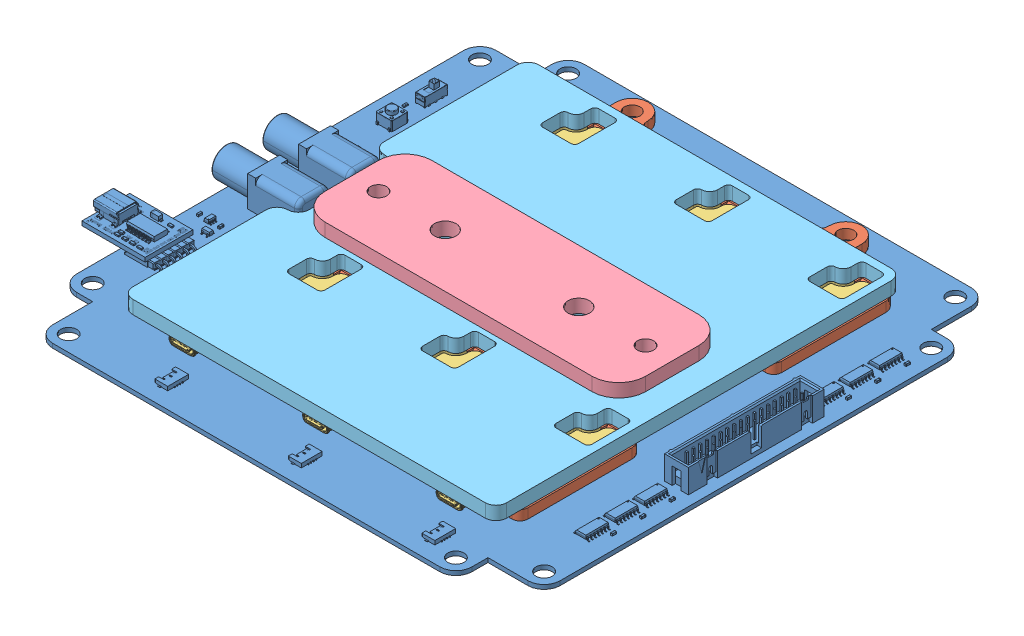
SolidWorks assembly Board Stage, configuration Default. Lengths in mm.
Overall size (202.87 18.85 190).
11 component instances, 5 part files, 12 mates.
Components (placement in the parent):
- Stage-1: Stage [Default] x (1 0 0) z (0 1 0) size (202.87 190 15.9)
- Board Bracket-1: Board Bracket [Default] at (95 0 -147) size (138 5.3 62)
- Board-1: Board [Default] at (29 3.7 -118) x (0 0 -1) z (0 -1 0) size (51.86 32.01 5.14)
- Board-2: Board [Default] at (79 3.7 -118) x (0 0 -1) z (0 -1 0) size (51.86 32.01 5.14)
- Board-3: Board [Default] at (129 3.7 -118) x (0 0 -1) z (0 -1 0) size (51.86 32.01 5.14)
- Board-4: Board [Default] at (29 3.7 -23) x (0 0 -1) z (0 -1 0) size (51.86 32.01 5.14)
- Board-5: Board [Default] at (79 3.7 -23) x (0 0 -1) z (0 -1 0) size (51.86 32.01 5.14)
- Board-6: Board [Default] at (129 3.7 -23) x (0 0 -1) z (0 -1 0) size (51.86 32.01 5.14)
- Board Bracket-2: Board Bracket [Default] at (95 0 -52) size (138 5.3 62)
- Board Clamp Top-2: Board Clamp Top [Default] at (95 10.3 -95) size (120 5 40)
- Board Clamp Bottom-2: Board Clamp Bottom [Default] at (95 5.3 -95) size (140 5 152)
Mates (geometry in assembly coordinates):
- Coincident3: coincident: plane of Board Bracket-1 through (95 3.7 -147) normal (0 1 0); plane of Board-1 through (39.5 3.7 -119) normal (0 -1 0)
- Concentric3: concentric: cylinder of Board Bracket-1 through (50 5.3 -164) axis (0 -1 0) radius 1; cylinder of Board-1 through (50 5.3252 -164) axis (0 -1 0) radius 1.05
- Concentric4: concentric: circle of Board Bracket-1; cylinder of Board-1 through (58 5.3252 -126) axis (0 -1 0) radius 1.05
- Concentric7: concentric: cylinder of Board Clamp Top-2 through (45 10.3 -95) axis (0 1 0) radius 3.05; cylinder of Board Clamp Bottom-2 through (45 5.3 -95) axis (0 1 0) radius 3.05
- Coincident7: coincident: plane of Board Clamp Top-2 through (95 10.3 -95) normal (0 -1 0); plane of Board Clamp Bottom-2 through (95 10.3 -95) normal (0 1 0)
- Concentric8: concentric: cylinder of Board Clamp Top-2 through (145 10.3 -95) axis (0 1 0) radius 3.05; cylinder of Board Clamp Bottom-2 through (145 5.3 -95) axis (0 1 0) radius 3.05
- Coincident8: coincident: plane of Board-4 through (39.5 5.3 -24) normal (0 1 0); plane of Board Clamp Bottom-2 through (95 5.3 -95) normal (0 -1 0)
- Coincident9: coincident: plane of Stage-1 through (6 0 -21) normal (0 1 0); plane of Board Bracket-1 through (95 0 -147) normal (0 -1 0)
- Concentric9: concentric: cylinder of Stage-1 through (55 -1.6 -180) axis (0 -1 0) radius 2.95; cylinder of Board Bracket-1 through (55 52.4032 -180) axis (0 -1 0) radius 2.95
- Concentric10: concentric: cylinder of Stage-1 through (135 -1.6 -180) axis (0 -1 0) radius 2.95; cylinder of Board Bracket-1 through (135 52.4032 -180) axis (0 -1 0) radius 2.95
- Concentric11: concentric: cylinder of Stage-1 through (70 -1.6 -95) axis (0 -1 0) radius 4.05; cylinder of Board Clamp Top-2 through (70 10.3 -95) axis (0 1 0) radius 4.05
- Concentric12: concentric: cylinder of Stage-1 through (120 -1.6 -95) axis (0 -1 0) radius 4.05; cylinder of Board Clamp Top-2 through (120 10.3 -95) axis (0 1 0) radius 4.05
